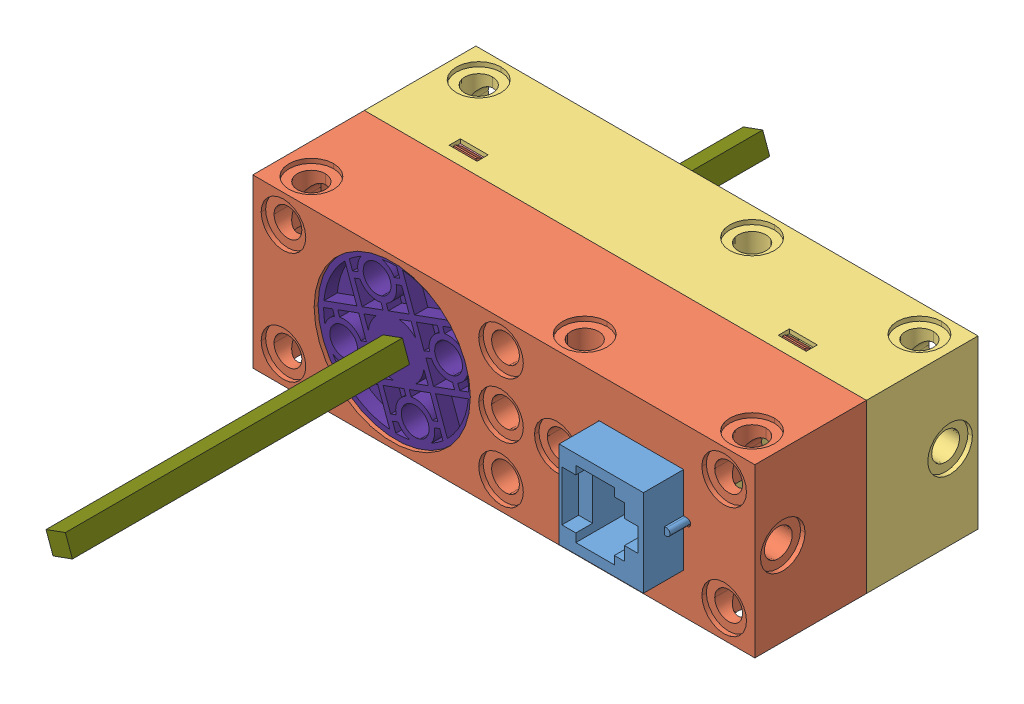
SolidWorks assembly 玩具装配体1_corrected, configuration Default. Lengths in mm.
Overall size (90 35.88 125).
33 component instances, 21 part files, 0 mates.
Components (placement in the parent):
- 玩具装配体1(2)^玩具装配体1_corrected-1: 玩具装配体1(2)^玩具装配体1_corrected [Default] at origin size (90 35.88 125) (virtual)
  - ____________ __^玩具装配体1(2)_玩具装配体1_corrected-1: ____________ __^玩具装配体1(2)_玩具装配体1_corrected [Default] at (8.1056 25.0507 26.4769) size (81.14 35.88 125) (virtual)
    - ________^____________ ___玩具装配体1(2)_玩具装配体1_corrected-1: ________^____________ ___玩具装配体1(2)_玩具装配体1_corrected [Default] at (-3.235 23.1684 17.3007) size (78 26.5 28.7) (virtual)
      - ________-1^_____________________ ___玩具装配体1(2)_玩具装配体1_corrected-1: ________-1^_____________________ ___玩具装配体1(2)_玩具装配体1_corrected [Default] at (79.0405 10.7038 66.7002) x (0 1 0) z (-1 0 0) size (20.4 28.41 40.6) (virtual)
        - 130____^________-1______________________ ___玩具装配体1(2)_玩具装配体1_corrected-1: 130____^________-1______________________ ___玩具装配体1(2)_玩具装配体1_corrected [Default] at (13.1972 32.2289 22.095) size (20.4 15.42 40.6) (virtual)
        - _________GearTrax^________-1______________________ ___玩具装配体1(2)_玩具装配体1_corrected-1: _________GearTrax^________-1______________________ ___玩具装配体1(2)_玩具装配体1_corrected [Default] at (13.1972 32.2289 60.0105) size (5.14 5.15 2.51) (virtual)
        - ______1^________-1______________________ ___玩具装配体1(2)_玩具装配体1_corrected-1: ______1^________-1______________________ ___玩具装配体1(2)_玩具装配体1_corrected [Default] at (13.1972 32.2289 21.695) x (-1 0 0) z (0 0 -1) size (19.6 28 0.8) (virtual)
      - ____^_____________________ ___玩具装配体1(2)_玩具装配体1_corrected-1: ____^_____________________ ___玩具装配体1(2)_玩具装配体1_corrected [Default] at (-11.0546 37.151 26.4713) size (43 26.5 17) (virtual)
      - ____-0^_____________________ ___玩具装配体1(2)_玩具装配体1_corrected-1: ____-0^_____________________ ___玩具装配体1(2)_玩具装配体1_corrected [Default] at (19.3454 23.901 27.4713) x (0.849881 -0.526974 0) z (0 0 1) size (2 2 17.3) (virtual)
    - __________^____________ ___玩具装配体1(2)_玩具装配体1_corrected-1: __________^____________ ___玩具装配体1(2)_玩具装配体1_corrected [Default] at (21.2756 42.8015 58.464) x (-0.874477 -0.485066 0) z (0 0 -1) size (21.33 21.33 6.2) (virtual)
      - Z13M0.6__6.2__^_______________________ ___玩具装配体1(2)_玩具装配体1_corrected-1: Z13M0.6__6.2__^_______________________ ___玩具装配体1(2)_玩具装配体1_corrected [Default] at (1173.14 3914.1005 3.992) size (9.48 9.54 6.2) (virtual)
      - _________GearTrax-1^_______________________ ___玩具装配体1(2)_玩具装配体1_corrected-1: _________GearTrax-1^_______________________ ___玩具装配体1(2)_玩具装配体1_corrected [Default] at (2.4466 6.2377 6.9147) x (-0.063071 0.998009 0) z (0 0 -1) size (20.1 20.11 1.51) (virtual)
    - ____22__38^____________ ___玩具装配体1(2)_玩具装配体1_corrected-1: ____22__38^____________ ___玩具装配体1(2)_玩具装配体1_corrected [Default] at (14.2004 56.9635 69.366) x (0.000452 -1 0) z (0 0 -1) size (23.9 23.96 6.2) (virtual)
      - Z38M0.6__2__^____22__38_____________ ___玩具装配体1(2)_玩具装配体1_corrected-1: Z38M0.6__2__^____22__38_____________ ___玩具装配体1(2)_玩具装配体1_corrected [Default] at (1346.5029 3922.186 16.084) size (23.9 23.96 2) (virtual)
      - Z22M0.6^____22__38_____________ ___玩具装配体1(2)_玩具装配体1_corrected-1: Z22M0.6^____22__38_____________ ___玩具装配体1(2)_玩具装配体1_corrected [Default] at (1192.4286 3849.0893 11.884) size (14.87 15 6.2) (virtual)
    - ____13__30^____________ ___玩具装配体1(2)_玩具装配体1_corrected-1: ____13__30^____________ ___玩具装配体1(2)_玩具装配体1_corrected [Default] at (10.1665 52.004 63.32) x (0.917069 0.398729 0) z (0 0 -1) size (18.53 18.6 5.5) (virtual)
      - Z13M0.6__5.5__^____13__30_____________ ___玩具装配体1(2)_玩具装配体1_corrected-1: Z13M0.6__5.5__^____13__30_____________ ___玩具装配体1(2)_玩具装配体1_corrected [Default] at (1248.1045 3738.5426 3.348) size (9.48 9.54 5.5) (virtual)
      - Z30M0.6^____13__30_____________ ___玩具装配体1(2)_玩具装配体1_corrected-1: Z30M0.6^____13__30_____________ ___玩具装配体1(2)_玩具装配体1_corrected [Default] at (1316.5243 3845.8896 6.848) size (18.53 18.6 2) (virtual)
    - Z38M0.6__18.9__^____________ ___玩具装配体1(2)_玩具装配体1_corrected-1: Z38M0.6__18.9__^____________ ___玩具装配体1(2)_玩具装配体1_corrected [Default] at (-156.8999 3954.1504 57.482) x (0.939862 0.341554 0) z (0 0 1) size (23.9 23.96 36.99) (virtual)
    - ____-2^____________ ___玩具装配体1(2)_玩具装配体1_corrected-1: ____-2^____________ ___玩具装配体1(2)_玩具装配体1_corrected [Default] at (-14.2896 33.8194 62.772) x (1 0 0) z (0 0 -1) size (43 26.5 18.5) (virtual)
    - ________-3^____________ ___玩具装配体1(2)_玩具装配体1_corrected-1: ________-3^____________ ___玩具装配体1(2)_玩具装配体1_corrected [Default] at (-11.2896 57.3194 61.772) x (0.644574 -0.764542 0) z (0 0 -1) size (3.8 3.8 14.01) (virtual)
    - ________-3^____________ ___玩具装配体1(2)_玩具装配体1_corrected-2: ________-3^____________ ___玩具装配体1(2)_玩具装配体1_corrected [Default] at (25.7104 57.3194 61.772) x (0.644574 -0.764542 0) z (0 0 -1) size (3.8 3.8 14.01) (virtual)
    - ________-3^____________ ___玩具装配体1(2)_玩具装配体1_corrected-3: ________-3^____________ ___玩具装配体1(2)_玩具装配体1_corrected [Default] at (25.7104 36.8194 61.772) x (0.644574 -0.764542 0) z (0 0 -1) size (3.8 3.8 14.01) (virtual)
    - ________-3^____________ ___玩具装配体1(2)_玩具装配体1_corrected-4: ________-3^____________ ___玩具装配体1(2)_玩具装配体1_corrected [Default] at (-11.2896 36.8194 61.772) x (0.644574 -0.764542 0) z (0 0 -1) size (3.8 3.8 14.01) (virtual)
    - ________-4^____________ ___玩具装配体1(2)_玩具装配体1_corrected-1: ________-4^____________ ___玩具装配体1(2)_玩具装配体1_corrected [Default] at (32.2104 53.2694 51.772) x (0 -0.340814 0.940131) z (-1 0 0) size (3.6 3.6 6.21) (virtual)
    - ________-4^____________ ___玩具装配体1(2)_玩具装配体1_corrected-2: ________-4^____________ ___玩具装配体1(2)_玩具装配体1_corrected [Default] at (32.2104 40.8694 51.772) x (0 -0.063636 0.997973) z (-1 0 0) size (3.6 3.6 6.21) (virtual)
    - ______^____________ ___玩具装配体1(2)_玩具装配体1_corrected-1: ______^____________ ___玩具装配体1(2)_玩具装配体1_corrected [Default] at (0.5104 47.0694 70.4668) x (0.939862 0.341554 0) z (0 0 1) size (3.7 3.7 125) (virtual)
    - ____-5^____________ ___玩具装配体1(2)_玩具装配体1_corrected-1: ____-5^____________ ___玩具装配体1(2)_玩具装配体1_corrected [Default] at (0.5104 47.0694 72.572) x (0 0 -1) z (0.939862 0.341554 0) size (8.4 28 28) (virtual)
    - ____-5^____________ ___玩具装配体1(2)_玩具装配体1_corrected-2: ____-5^____________ ___玩具装配体1(2)_玩具装配体1_corrected [Default] at (0.5104 47.0694 33.582) x (0 0 1) z (-0.939862 -0.341554 0) size (8.4 28 28) (virtual)
    - ____-6^____________ ___玩具装配体1(2)_玩具装配体1_corrected-1: ____-6^____________ ___玩具装配体1(2)_玩具装配体1_corrected [Default] at (59.6947 47.0694 51.772) x (0 0.059635 0.99822) z (-1 0 0) size (14 14 5.5) (virtual)
    - RJ45______^____________ ___玩具装配体1(2)_玩具装配体1_corrected-1: RJ45______^____________ ___玩具装配体1(2)_玩具装配体1_corrected [Default] at (53.7104 47.0971 80.432) x (0 0 1) z (0 -1 0) size (20.96 20.45 15.62) (virtual)
  - ____1^玩具装配体1(2)_玩具装配体1_corrected-1: ____1^玩具装配体1(2)_玩具装配体1_corrected [Default] at (28.616 72.1201 99.7488) x (1 0 0) z (0 0 -1) size (90 30 24) (virtual)
  - ____2^玩具装配体1(2)_玩具装配体1_corrected-1: ____2^玩具装配体1(2)_玩具装配体1_corrected [Default] at (28.616 72.1201 59.7488) size (90 30 20) (virtual)
